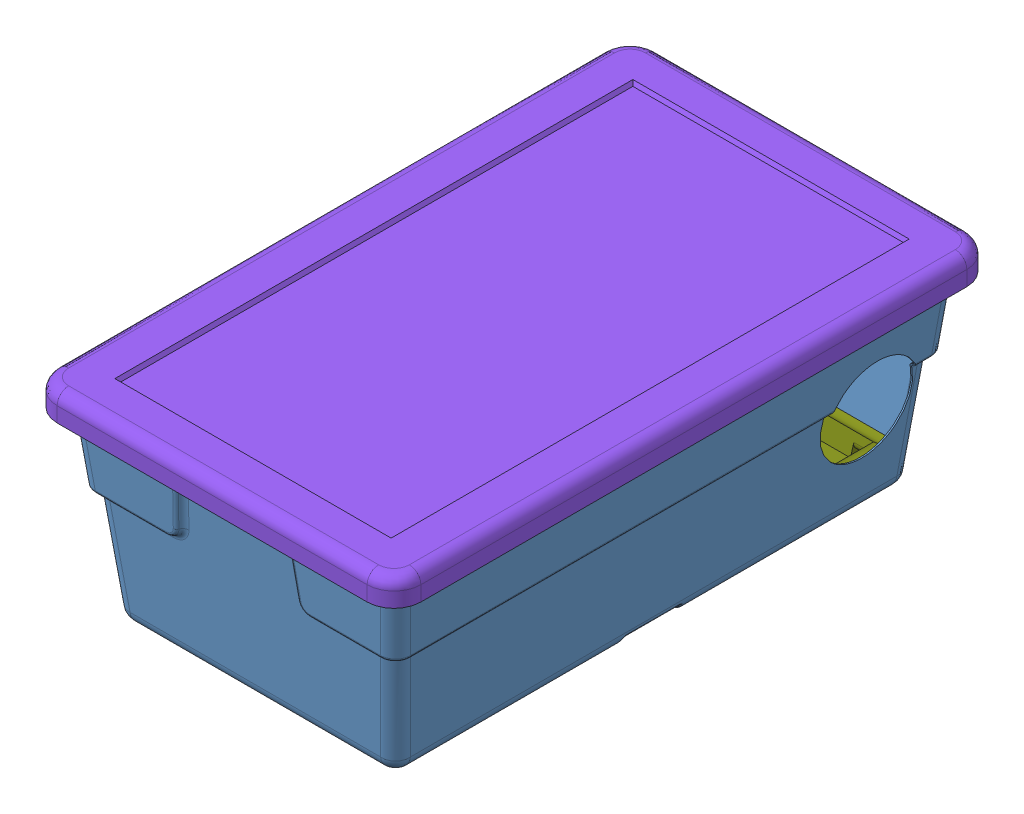
SolidWorks assembly electronics_box, configuration Default. Lengths in mm.
Overall size (200.66 116.21 330.83).
278 component instances, 62 part files, 7 mates.
Components (placement in the parent):
- sterilite_box-1: sterilite_box [Default] at (6.4065 -41.9824 -170.8478) size (195.22 114.3 325.39)
- electronics_tray-1: electronics_tray [Default] at (67.0566 -75.9526 -72.8113) x (0 0 1) z (-1 0 0) size (203.2 36.13 152.4)
  - ibt2_assembly-1: ibt2_assembly [Default] at (25.1982 40.7289 22.1019) size (49.66 21.28 49.78)
    - IBT2_pcb-1: IBT2_pcb [Default] at (-57.2691 7.2367 24.7687) size (49.66 1.57 49.4)
    - header_male_2x4-1: header_male_2x4 [Default] at (4.8115 23.0826 24.5335) x (1 0 0) z (0 -1 0) size (10.16 5.08 10.92)
      - header_pin_base_2x4-1: header_pin_base_2x4 [Default] at (-49.9521 21.6346 11.7311) size (10.16 5.08 2.54)
      - header_pin-1: header_pin [Default] at (-56.3021 22.9046 6.0161) size (0.64 0.64 10.92)
      - header_pin-2: header_pin [Default] at (-56.3021 20.3646 6.0161) size (0.64 0.64 10.92)
      - header_pin-3: header_pin [Default] at (-53.7621 22.9046 6.0161) size (0.64 0.64 10.92)
      - header_pin-4: header_pin [Default] at (-53.7621 20.3646 6.0161) size (0.64 0.64 10.92)
      - header_pin-5: header_pin [Default] at (-51.2221 22.9046 6.0161) size (0.64 0.64 10.92)
      - header_pin-6: header_pin [Default] at (-51.2221 20.3646 6.0161) size (0.64 0.64 10.92)
      - header_pin-7: header_pin [Default] at (-48.6821 22.9046 6.0161) size (0.64 0.64 10.92)
      - header_pin-8: header_pin [Default] at (-48.6821 20.3646 6.0161) size (0.64 0.64 10.92)
    - AMP_screw-terminal_2POS_large-1: AMP_screw-terminal_2POS_large [Default] at (-57.2056 17.0115 0.4662) x (-1 0 0) z (0 0 -1) size (10.66 17 9)
    - AMP_screw-terminal_2POS_large-2: AMP_screw-terminal_2POS_large [Default] at (-47.0456 17.0115 0.4662) x (-1 0 0) z (0 0 -1) size (10.66 17 9)
    - cap_5mm_pitch-1: cap_5mm_pitch [Default] at (-68.3924 8.8115 4.7662) size (10.16 19.69 10.16)
    - d2pak-1: d2pak [Default] at (-63.2409 8.7779 25.6248) x (1 0 0) z (0 0.999978 0.006671) size (9.87 15.09 4.26)
    - d2pak-2: d2pak [Default] at (-52.336 8.7779 25.6248) x (1 0 0) z (0 0.999978 0.006671) size (9.87 15.09 4.26)
    - SOIC20 wide-1: SOIC20 wide [Default] at (-39.9304 8.5615 36.0347) x (1 0 0) z (0 1 0) size (13 10.17 2.01)
    - cap_0805-1: cap_0805 [Default] at (-38.0286 9.3449 27.3468) x (1 0 0) z (0 -1 0) size (2.03 1.32 0.56)
    - resistor_0805-1: resistor_0805 [Default] at (-48.3156 9.3449 41.6216) x (0 0 -1) z (0 -1 0) size (2.03 1.32 0.56)
    - resistor_0805-2: resistor_0805 [Default] at (-50.4517 9.3449 41.6216) x (0 0 -1) z (0 -1 0) size (2.03 1.32 0.56)
    - resistor_0805-3: resistor_0805 [Default] at (-52.5879 9.3449 41.6216) x (0 0 -1) z (0 -1 0) size (2.03 1.32 0.56)
    - resistor_0805-4: resistor_0805 [Default] at (-54.724 9.3449 41.6216) x (0 0 -1) z (0 -1 0) size (2.03 1.32 0.56)
    - resistor_0805-5: resistor_0805 [Default] at (-56.8602 9.3449 41.6216) x (0 0 -1) z (0 -1 0) size (2.03 1.32 0.56)
    - resistor_0805-6: resistor_0805 [Default] at (-58.9963 9.3449 41.6216) x (0 0 -1) z (0 -1 0) size (2.03 1.32 0.56)
    - resistor_0805-7: resistor_0805 [Default] at (-61.1324 9.3449 41.6216) x (0 0 -1) z (0 -1 0) size (2.03 1.32 0.56)
    - resistor_0805-8: resistor_0805 [Default] at (-63.2686 9.3449 41.6216) x (0 0 -1) z (0 -1 0) size (2.03 1.32 0.56)
  - ibt2_assembly-2: ibt2_assembly [Default] at (-89.34 40.7289 121.0422) x (-1 0 0) z (0 0 -1) size (49.66 21.28 49.78)
    - IBT2_pcb-1: IBT2_pcb [Default] at (-57.2691 7.2367 24.7687) size (49.66 1.57 49.4)
    - header_male_2x4-1: header_male_2x4 [Default] at (4.8115 23.0826 24.5335) x (1 0 0) z (0 -1 0) size (10.16 5.08 10.92)
      - header_pin_base_2x4-1: header_pin_base_2x4 [Default] at (-49.9521 21.6346 11.7311) size (10.16 5.08 2.54)
      - header_pin-1: header_pin [Default] at (-56.3021 22.9046 6.0161) size (0.64 0.64 10.92)
      - header_pin-2: header_pin [Default] at (-56.3021 20.3646 6.0161) size (0.64 0.64 10.92)
      - header_pin-3: header_pin [Default] at (-53.7621 22.9046 6.0161) size (0.64 0.64 10.92)
      - header_pin-4: header_pin [Default] at (-53.7621 20.3646 6.0161) size (0.64 0.64 10.92)
      - header_pin-5: header_pin [Default] at (-51.2221 22.9046 6.0161) size (0.64 0.64 10.92)
      - header_pin-6: header_pin [Default] at (-51.2221 20.3646 6.0161) size (0.64 0.64 10.92)
      - header_pin-7: header_pin [Default] at (-48.6821 22.9046 6.0161) size (0.64 0.64 10.92)
      - header_pin-8: header_pin [Default] at (-48.6821 20.3646 6.0161) size (0.64 0.64 10.92)
    - AMP_screw-terminal_2POS_large-1: AMP_screw-terminal_2POS_large [Default] at (-57.2056 17.0115 0.4662) x (-1 0 0) z (0 0 -1) size (10.66 17 9)
    - AMP_screw-terminal_2POS_large-2: AMP_screw-terminal_2POS_large [Default] at (-47.0456 17.0115 0.4662) x (-1 0 0) z (0 0 -1) size (10.66 17 9)
    - cap_5mm_pitch-1: cap_5mm_pitch [Default] at (-68.3924 8.8115 4.7662) size (10.16 19.69 10.16)
    - d2pak-1: d2pak [Default] at (-63.2409 8.7779 25.6248) x (1 0 0) z (0 0.999978 0.006671) size (9.87 15.09 4.26)
    - d2pak-2: d2pak [Default] at (-52.336 8.7779 25.6248) x (1 0 0) z (0 0.999978 0.006671) size (9.87 15.09 4.26)
    - SOIC20 wide-1: SOIC20 wide [Default] at (-39.9304 8.5615 36.0347) x (1 0 0) z (0 1 0) size (13 10.17 2.01)
    - cap_0805-1: cap_0805 [Default] at (-38.0286 9.3449 27.3468) x (1 0 0) z (0 -1 0) size (2.03 1.32 0.56)
    - resistor_0805-1: resistor_0805 [Default] at (-48.3156 9.3449 41.6216) x (0 0 -1) z (0 -1 0) size (2.03 1.32 0.56)
    - resistor_0805-2: resistor_0805 [Default] at (-50.4517 9.3449 41.6216) x (0 0 -1) z (0 -1 0) size (2.03 1.32 0.56)
    - resistor_0805-3: resistor_0805 [Default] at (-52.5879 9.3449 41.6216) x (0 0 -1) z (0 -1 0) size (2.03 1.32 0.56)
    - resistor_0805-4: resistor_0805 [Default] at (-54.724 9.3449 41.6216) x (0 0 -1) z (0 -1 0) size (2.03 1.32 0.56)
    - resistor_0805-5: resistor_0805 [Default] at (-56.8602 9.3449 41.6216) x (0 0 -1) z (0 -1 0) size (2.03 1.32 0.56)
    - resistor_0805-6: resistor_0805 [Default] at (-58.9963 9.3449 41.6216) x (0 0 -1) z (0 -1 0) size (2.03 1.32 0.56)
    - resistor_0805-7: resistor_0805 [Default] at (-61.1324 9.3449 41.6216) x (0 0 -1) z (0 -1 0) size (2.03 1.32 0.56)
    - resistor_0805-8: resistor_0805 [Default] at (-63.2686 9.3449 41.6216) x (0 0 -1) z (0 -1 0) size (2.03 1.32 0.56)
  - Arduino_mega-1: Arduino_mega [Default] at (5.4045 37.4555 130.5264) x (0 0 1) z (0 1 0) size (107.7 53.34 12.38)
    - Arduino_mega-1: Arduino_mega [Default] at (-98.4513 -6.297 10.51) size (101.6 53.34 1.59)
    - USB-jack-1: USB-jack [Default] at (-104.5473 25.6308 12.0975) size (16.46 12.14 10.79)
    - DC-jack-1: DC-jack [Default] at (-99.9245 -2.5632 12.0975) x (0 1 0) z (0 0 -1) size (8.79 13.59 10.72)
    - header_8-pin-1: header_8-pin [Default] at (-53.7727 -5.0778 12.0975) size (20.32 2.54 8.56)
    - header_8-pin-2: header_8-pin [Default] at (-30.6587 -5.0778 12.0975) size (20.32 2.54 8.56)
    - header_8-pin-3: header_8-pin [Default] at (-8.0781 -5.0778 12.0975) size (20.32 2.54 8.56)
    - header_8-pin-4: header_8-pin [Default] at (-35.7895 43.0044 12.0975) size (20.32 2.54 8.56)
    - header_8-pin-5: header_8-pin [Default] at (-13.1835 43.0044 12.0975) size (20.32 2.54 8.56)
    - header_10-pin-1: header_10-pin [Default] at (-58.0145 43.0044 12.0975) size (25.4 2.54 8.56)
    - header_36-pin-1: header_36-pin [Default] at (-0.5343 43.0298 12.0975) x (0 1 0) z (0 0 1) size (45.72 5.08 8.56)
  - arduino uno-1: arduino uno [Default] at (57.5276 49.6156 28.9001) x (-1 0 0) z (0 0 -1) size (53.34 15.25 74.97)
    - unoboard blue-1: unoboard blue [Default] at origin size (53.34 1.65 68.58)
    - 47uf CAP Dcase-1: 47uf CAP Dcase [Default] at (-9.4141 0 -18.4991) x (0 0 -1) z (1 0 0) size (6.6 5.81 8)
    - USB type b-1: USB type b [Default] at (-38.02 0.43 6.35) size (13.72 15.2 16.54)
      - USB SHELL-1: USB SHELL [Default] at origin size (13.72 15.2 16.54)
      - USB core-1: USB core [Default] at origin size (11.3 10.68 15.75)
      - usb top contact-1: usb top contact [Default] at (1.25 6.09 -0.38) size (1 9.67 13.76)
      - usb btm contact-1: usb btm contact [Default] at (1.25 4.41 -0.38) size (1 6.84 11.76)
      - usb btm contact-2: usb btm contact [Default] at (-1.25 4.41 -0.38) size (1 6.84 11.76)
      - usb top contact-2: usb top contact [Default] at (-1.25 6.09 -0.38) size (1 9.67 13.76)
    - power jack-1: power jack [Default] at (-7.675 0 1.905) size (11.2 15.2 15.9)
    - 47uf CAP Dcase-2: 47uf CAP Dcase [Default] at (-9.4141 0 -25.7132) x (0 0 -1) z (1 0 0) size (6.6 5.81 8)
    - crystal-1: crystal [Default] at (-26.162 0 -18.923) x (1 0 0) z (0 0 -1) size (4 5 11)
    - 2pin_header__02-1: 2pin_header__02 [Default] at (-46.23 0 -15.75) size (5 11.75 2.54)
    - nano - reg-1: nano - reg [Default] at (-17.399 0 -7.747) size (6.5 1.69 8.3)
    - led-1: led [Default] at (-34.29 0 -27.94) x (0 0 1) z (-1 0 0) size (4 0.86 1.35)
    - 2pin_header__02-2: 2pin_header__02 [Default] at (-30.43 0 -64.91) x (0 0 1) z (-1 0 0) size (5 11.75 2.54)
    - dip28-1: dip28 [Default] at (-16.383 1.5 -46.355) x (0 0 -1) z (1 0 0) size (35.48 7.37 10.1)
      - dip28-1: dip28 [Default] at origin size (35.48 2.8 10.1)
      - dip socket pin-1: dip socket pin [Default] at (16.51 2.8 -3.81) size (1.7 7.37 1.7)
      - dip socket pin-2: dip socket pin [Default] at (16.51 2.8 3.81) size (1.7 7.37 1.7)
      - dip socket pin-3: dip socket pin [Default] at (13.97 2.8 -3.81) size (1.7 7.37 1.7)
      - dip socket pin-4: dip socket pin [Default] at (13.97 2.8 3.81) size (1.7 7.37 1.7)
      - dip socket pin-5: dip socket pin [Default] at (11.43 2.8 -3.81) size (1.7 7.37 1.7)
      - dip socket pin-6: dip socket pin [Default] at (11.43 2.8 3.81) size (1.7 7.37 1.7)
      - dip socket pin-7: dip socket pin [Default] at (8.89 2.8 -3.81) size (1.7 7.37 1.7)
      - dip socket pin-8: dip socket pin [Default] at (8.89 2.8 3.81) size (1.7 7.37 1.7)
      - dip socket pin-9: dip socket pin [Default] at (6.35 2.8 -3.81) size (1.7 7.37 1.7)
      - dip socket pin-10: dip socket pin [Default] at (6.35 2.8 3.81) size (1.7 7.37 1.7)
      - dip socket pin-11: dip socket pin [Default] at (3.81 2.8 -3.81) size (1.7 7.37 1.7)
      - dip socket pin-12: dip socket pin [Default] at (3.81 2.8 3.81) size (1.7 7.37 1.7)
      - dip socket pin-13: dip socket pin [Default] at (1.27 2.8 -3.81) size (1.7 7.37 1.7)
      - dip socket pin-14: dip socket pin [Default] at (1.27 2.8 3.81) size (1.7 7.37 1.7)
      - dip socket pin-15: dip socket pin [Default] at (-1.27 2.8 -3.81) size (1.7 7.37 1.7)
      - dip socket pin-16: dip socket pin [Default] at (-1.27 2.8 3.81) size (1.7 7.37 1.7)
      - dip socket pin-17: dip socket pin [Default] at (-3.81 2.8 -3.81) size (1.7 7.37 1.7)
      - dip socket pin-18: dip socket pin [Default] at (-3.81 2.8 3.81) size (1.7 7.37 1.7)
      - dip socket pin-19: dip socket pin [Default] at (-6.35 2.8 -3.81) size (1.7 7.37 1.7)
      - dip socket pin-20: dip socket pin [Default] at (-6.35 2.8 3.81) size (1.7 7.37 1.7)
      - dip socket pin-21: dip socket pin [Default] at (-8.89 2.8 -3.81) size (1.7 7.37 1.7)
      - dip socket pin-22: dip socket pin [Default] at (-8.89 2.8 3.81) size (1.7 7.37 1.7)
      - dip socket pin-23: dip socket pin [Default] at (-11.43 2.8 -3.81) size (1.7 7.37 1.7)
      - dip socket pin-24: dip socket pin [Default] at (-11.43 2.8 3.81) size (1.7 7.37 1.7)
      - dip socket pin-25: dip socket pin [Default] at (-13.97 2.8 -3.81) size (1.7 7.37 1.7)
      - dip socket pin-26: dip socket pin [Default] at (-13.97 2.8 3.81) size (1.7 7.37 1.7)
      - dip socket pin-27: dip socket pin [Default] at (-16.51 2.8 -3.81) size (1.7 7.37 1.7)
      - dip socket pin-28: dip socket pin [Default] at (-16.51 2.8 3.81) size (1.7 7.37 1.7)
    - 2pin_header__02-3: 2pin_header__02 [Default] at (-27.89 0 -64.91) x (0 0 1) z (-1 0 0) size (5 11.75 2.54)
    - 2pin_header__02-4: 2pin_header__02 [Default] at (-25.35 0 -64.91) x (0 0 1) z (-1 0 0) size (5 11.75 2.54)
    - 2pin_header__02-5: 2pin_header__02 [Default] at (-46.23 0 -18.29) size (5 11.75 2.54)
    - 2pin_header__02-6: 2pin_header__02 [Default] at (-46.23 0 -20.83) size (5 11.75 2.54)
    - atmega16u2-1: atmega16u2 [Default] at (-34.671 0.06 -20) x (1 0 0) z (0 0 -1) size (5.5 1.01 5.5)
    - led-2: led [Default] at (-36.83 0 -27.94) x (0 0 1) z (-1 0 0) size (4 0.86 1.35)
    - led-3: led [Default] at (-42.037 0 -27.94) x (0 0 1) z (-1 0 0) size (4 0.86 1.35)
    - led-4: led [Default] at (-36.576 0 -58.42) x (0 0 1) z (-1 0 0) size (4 0.86 1.35)
    - 8 PORT HEADER-3: 8 PORT HEADER [Default] at (-50.8 0 -45.72) x (0 0 -1) z (1 0 0) size (20.32 10.51 2.41)
    - 8 PORT HEADER-4: 8 PORT HEADER [Default] at (-2.54 0 -27.94) x (0 0 -1) z (1 0 0) size (20.32 10.51 2.41)
    - 6 PORT HEADER-3: 6 PORT HEADER [Default] at (-2.54 0 -50.8) x (0 0 -1) z (1 0 0) size (15.24 10.51 2.41)
    - 10 PORT HEADER-1: 10 PORT HEADER [Default] at (-50.8 0 -18.796) x (0 0 -1) z (1 0 0) size (25.4 10.51 2.41)
    - ATMEL328P-1: ATMEL328P [Default] at (-16.383 4.3 -46.355) x (0 0 -1) z (1 0 0) size (35 7.27 7.87)
    - 102 RESISTOR PACK-1: 102 RESISTOR PACK [Default] at (-33.782 0 -58.42) size (3.2 0.46 3)
    - 102 RESISTOR PACK-2: 102 RESISTOR PACK [Default] at (-39.37 0 -27.94) size (3.2 0.46 3)
    - 103 RESISTOR PACK-3: 103 RESISTOR PACK [Default] at (-23.876 0 -27.94) size (3.2 0.46 3)
    - 220 RESISTOR PACK-1: 220 RESISTOR PACK [Default] at (-36.83 0 -12.827) size (3.2 0.46 3)
    - 16mhz crystal - measured-1: 16mhz crystal - measured [Default] at (-24.892 0 -41.275) x (0 0 -1) z (1 0 0) size (3.4 0.8 2)
    - PADS001-1: PADS001 [Default] at (-39.878 0.1 -18.288) x (-1 0 0) z (0 0 1) size (4.54 0.1 4.54)
    - 603 cap on pad-1: 603 cap on pad [Default] at (-44.45 0 -27.94) x (0 0 -1) z (1 0 0) size (2.76 0.9 1.12)
    - ssot3-1: ssot3 [Default] at (-26.5 0 -8.128) x (-1 0 0) z (0 0 -1) size (3 1.13 3.09)
    - mf-msmf050-2-1: mf-msmf050-2 [Default] at (-26.5 0 -4.064) size (5.77 1.02 3.72)
    - 603 cap on pad-2: 603 cap on pad [Default] at (-29.845 0 -27.94) x (0 0 -1) z (1 0 0) size (2.76 0.9 1.12)
    - 603 cap on pad-3: 603 cap on pad [Default] at (-31.496 0 -27.94) x (0 0 -1) z (1 0 0) size (2.76 0.9 1.12)
    - lmv358-1: lmv358 [Default] at (-15.24 0 -21.971) x (0 0 -1) z (1 0 0) size (3.7 1.4 2.9)
    - 603 cap on pad-4: 603 cap on pad [Default] at (-15.24 0 -18.415) size (2.76 0.9 1.12)
    - 603 cap on pad-5: 603 cap on pad [Default] at (-29.845 0 -12.065) x (0 0 1) z (-1 0 0) size (2.76 0.9 1.12)
    - 603 cap on pad-6: 603 cap on pad [Default] at (-29.591 0 -22.352) x (0 0 1) z (-1 0 0) size (2.76 0.9 1.12)
    - 603 cap on pad-7: 603 cap on pad [Default] at (-29.591 0 -16.002) x (0 0 1) z (-1 0 0) size (2.76 0.9 1.12)
    - 603 cap on pad-8: 603 cap on pad [Default] at (-41.91 0 -12.7) x (0 0 1) z (-1 0 0) size (2.76 0.9 1.12)
    - lp2985dgkr-1: lp2985dgkr [Default] at (-20.32 0 -19.05) x (0 0 -1) z (1 0 0) size (5.85 1.1 3)
    - cd1206 diode-1: cd1206 diode [Default] at (-27.94 0 -59.436) x (0 0 -1) z (1 0 0) size (2.07 0.96 5)
    - cd1206 diode-2: cd1206 diode [Default] at (-46.228 0 -13.081) x (0 0 1) z (-1 0 0) size (2.07 0.96 5)
    - 603 resistor-1: 603 resistor [Default] at (-29.591 0 -19.05) x (0 0 1) z (-1 0 0) size (2.36 0.61 1.03)
    - blm21-1: blm21 [Default] at (-45.085 0 -7.62) x (0 0 -1) z (1 0 0) size (2.76 0.95 1.32)
    - m7 diode-1: m7 diode [Default] at (-2.794 0 -21.59) x (0 0 -1) z (1 0 0) size (6.66 2.35 2.5)
    - MLC0603-1: MLC0603 [Default] at (-33.655 0 -12.827) x (0 0 -1) z (1 0 0) size (2.36 0.6 1.03)
    - MLC0603-2: MLC0603 [Default] at (-39.37 0 -12.827) x (0 0 -1) z (1 0 0) size (2.36 0.6 1.03)
    - RESET BUTTON-1: RESET BUTTON [Default] at (-49.403 0 -6.35) size (6.2 3.1 9.6)
      - RESET CORE-1: RESET CORE [Default] at (0 0.1 0) x (-1 0 0) z (0 0 -1) size (6.2 3.1 9.6)
      - RESET-1: RESET [Default] at (0 0.1 0) x (0 0 1) z (-1 0 0) size (7.3 2 6.2)
    - 603 cap on pad-9: 603 cap on pad [Default] at (-15.24 0 -25.625) size (2.76 0.9 1.12)
  - electronics_tray_tray-1: electronics_tray_tray [Default] at origin size (203.2 13.95 152.4)
  - m3x6mm_cap_screw-1: m3x6mm_cap_screw [92095A179] at (-11.9414 51.1904 27.3507) x (-0.837169 0 -0.546944) z (0 1 0) size (5.7 5.7 7.77)
  - bms_assembly-1: bms_assembly [Default] at (83.3041 41.8308 46.3558) x (0 0 -1) z (0 1 0) size (88.9 53.34 22.95)
    - bms_board-1: bms_board [Default] at (-80.72 -27.381 18.8348) size (88.9 53.34 1.57)
    - AMP_screw-terminal_2POS_large-1: AMP_screw-terminal_2POS_large [Default] at (-79.94 10.719 28.6096) x (0 -1 0) z (-1 0 0) size (10.66 17 9)
    - AMP_screw-terminal_2POS_large-2: AMP_screw-terminal_2POS_large [Default] at (-79.94 0.559 28.6096) x (0 -1 0) z (-1 0 0) size (10.66 17 9)
    - B4B-XH-Apart-1: B4B-XH-Apart [Default] at (-77.791 -14.995 20.4096) x (0 1 0) z (1 0 0) size (12.4 10.4 5.75)
    - header_male_1x10-1: header_male_1x10 [Default] at (49.0022 32.4877 36.1995) x (0 1 0) z (0 0 1) size (2.54 25.4 10.92)
      - header_pin-1: header_pin [Default] at (-57.3287 73.639 -25.2387) size (0.64 0.64 10.92)
      - header_pin_base_single-1: header_pin_base_single [Default] at (-58.5987 72.369 -19.9047) size (2.54 2.54 2.54)
      - header_pin_base_single-2: header_pin_base_single [Default] at (-58.5987 69.829 -19.9047) size (2.54 2.54 2.54)
      - header_pin_base_single-3: header_pin_base_single [Default] at (-58.5987 67.289 -19.9047) size (2.54 2.54 2.54)
      - header_pin_base_single-4: header_pin_base_single [Default] at (-58.5987 64.749 -19.9047) size (2.54 2.54 2.54)
      - header_pin_base_single-5: header_pin_base_single [Default] at (-58.5987 62.209 -19.9047) size (2.54 2.54 2.54)
      - header_pin_base_single-6: header_pin_base_single [Default] at (-58.5987 59.669 -19.9047) size (2.54 2.54 2.54)
      - header_pin-2: header_pin [Default] at (-57.3287 71.099 -25.2387) size (0.64 0.64 10.92)
      - header_pin-3: header_pin [Default] at (-57.3287 68.559 -25.2387) size (0.64 0.64 10.92)
      - header_pin-4: header_pin [Default] at (-57.3287 66.019 -25.2387) size (0.64 0.64 10.92)
      - header_pin-5: header_pin [Default] at (-57.3287 63.479 -25.2387) size (0.64 0.64 10.92)
      - header_pin-6: header_pin [Default] at (-57.3287 60.939 -25.2387) size (0.64 0.64 10.92)
      - header_pin-7: header_pin [Default] at (-57.3287 58.399 -25.2387) size (0.64 0.64 10.92)
      - header_pin-8: header_pin [Default] at (-57.3287 55.859 -25.2387) size (0.64 0.64 10.92)
      - header_pin_base_single-7: header_pin_base_single [Default] at (-58.5987 57.129 -19.9047) size (2.54 2.54 2.54)
      - header_pin_base_single-8: header_pin_base_single [Default] at (-58.5987 54.589 -19.9047) size (2.54 2.54 2.54)
      - header_pin_base_single-9: header_pin_base_single [Default] at (-58.5987 52.049 -19.9047) size (2.54 2.54 2.54)
      - header_pin_base_single-10: header_pin_base_single [Default] at (-58.5987 49.509 -19.9047) size (2.54 2.54 2.54)
      - header_pin-9: header_pin [Default] at (-57.3287 53.319 -25.2387) size (0.64 0.64 10.92)
      - header_pin-10: header_pin [Default] at (-57.3287 50.779 -25.2387) size (0.64 0.64 10.92)
    - header_male_1x8-1: header_male_1x8 [Default] at (-84.3058 -33.9097 36.1995) x (0 -1 0) z (0 0 1) size (2.54 20.32 10.92)
      - header_pin-1: header_pin [Default] at (-57.3287 73.639 -25.2387) size (0.64 0.64 10.92)
      - header_pin_base_single-1: header_pin_base_single [Default] at (-58.5987 72.369 -19.9047) size (2.54 2.54 2.54)
      - header_pin_base_single-2: header_pin_base_single [Default] at (-58.5987 69.829 -19.9047) size (2.54 2.54 2.54)
      - header_pin_base_single-3: header_pin_base_single [Default] at (-58.5987 67.289 -19.9047) size (2.54 2.54 2.54)
      - header_pin_base_single-4: header_pin_base_single [Default] at (-58.5987 64.749 -19.9047) size (2.54 2.54 2.54)
      - header_pin_base_single-5: header_pin_base_single [Default] at (-58.5987 62.209 -19.9047) size (2.54 2.54 2.54)
      - header_pin_base_single-6: header_pin_base_single [Default] at (-58.5987 59.669 -19.9047) size (2.54 2.54 2.54)
      - header_pin-2: header_pin [Default] at (-57.3287 71.099 -25.2387) size (0.64 0.64 10.92)
      - header_pin-3: header_pin [Default] at (-57.3287 68.559 -25.2387) size (0.64 0.64 10.92)
      - header_pin-4: header_pin [Default] at (-57.3287 66.019 -25.2387) size (0.64 0.64 10.92)
      - header_pin-5: header_pin [Default] at (-57.3287 63.479 -25.2387) size (0.64 0.64 10.92)
      - header_pin-6: header_pin [Default] at (-57.3287 60.939 -25.2387) size (0.64 0.64 10.92)
      - header_pin-7: header_pin [Default] at (-57.3287 58.399 -25.2387) size (0.64 0.64 10.92)
      - header_pin-8: header_pin [Default] at (-57.3287 55.859 -25.2387) size (0.64 0.64 10.92)
      - header_pin_base_single-7: header_pin_base_single [Default] at (-58.5987 57.129 -19.9047) size (2.54 2.54 2.54)
      - header_pin_base_single-8: header_pin_base_single [Default] at (-58.5987 54.589 -19.9047) size (2.54 2.54 2.54)
    - header_male_1x8-2: header_male_1x8 [Default] at (-102.0858 -82.1697 36.1995) x (0 -1 0) z (0 0 1) size (2.54 20.32 10.92)
      - header_pin-1: header_pin [Default] at (-57.3287 73.639 -25.2387) size (0.64 0.64 10.92)
      - header_pin_base_single-1: header_pin_base_single [Default] at (-58.5987 72.369 -19.9047) size (2.54 2.54 2.54)
      - header_pin_base_single-2: header_pin_base_single [Default] at (-58.5987 69.829 -19.9047) size (2.54 2.54 2.54)
      - header_pin_base_single-3: header_pin_base_single [Default] at (-58.5987 67.289 -19.9047) size (2.54 2.54 2.54)
      - header_pin_base_single-4: header_pin_base_single [Default] at (-58.5987 64.749 -19.9047) size (2.54 2.54 2.54)
      - header_pin_base_single-5: header_pin_base_single [Default] at (-58.5987 62.209 -19.9047) size (2.54 2.54 2.54)
      - header_pin_base_single-6: header_pin_base_single [Default] at (-58.5987 59.669 -19.9047) size (2.54 2.54 2.54)
      - header_pin-2: header_pin [Default] at (-57.3287 71.099 -25.2387) size (0.64 0.64 10.92)
      - header_pin-3: header_pin [Default] at (-57.3287 68.559 -25.2387) size (0.64 0.64 10.92)
      - header_pin-4: header_pin [Default] at (-57.3287 66.019 -25.2387) size (0.64 0.64 10.92)
      - header_pin-5: header_pin [Default] at (-57.3287 63.479 -25.2387) size (0.64 0.64 10.92)
      - header_pin-6: header_pin [Default] at (-57.3287 60.939 -25.2387) size (0.64 0.64 10.92)
      - header_pin-7: header_pin [Default] at (-57.3287 58.399 -25.2387) size (0.64 0.64 10.92)
      - header_pin-8: header_pin [Default] at (-57.3287 55.859 -25.2387) size (0.64 0.64 10.92)
      - header_pin_base_single-7: header_pin_base_single [Default] at (-58.5987 57.129 -19.9047) size (2.54 2.54 2.54)
      - header_pin_base_single-8: header_pin_base_single [Default] at (-58.5987 54.589 -19.9047) size (2.54 2.54 2.54)
    - header_male_1x6-1: header_male_1x6 [Default] at (27.4122 80.7477 36.1995) x (0 1 0) z (0 0 1) size (2.54 15.24 10.92)
      - header_pin-1: header_pin [Default] at (-57.3287 73.639 -25.2387) size (0.64 0.64 10.92)
      - header_pin_base_single-1: header_pin_base_single [Default] at (-58.5987 72.369 -19.9047) size (2.54 2.54 2.54)
      - header_pin_base_single-2: header_pin_base_single [Default] at (-58.5987 69.829 -19.9047) size (2.54 2.54 2.54)
      - header_pin_base_single-3: header_pin_base_single [Default] at (-58.5987 67.289 -19.9047) size (2.54 2.54 2.54)
      - header_pin_base_single-4: header_pin_base_single [Default] at (-58.5987 64.749 -19.9047) size (2.54 2.54 2.54)
      - header_pin_base_single-5: header_pin_base_single [Default] at (-58.5987 62.209 -19.9047) size (2.54 2.54 2.54)
      - header_pin_base_single-6: header_pin_base_single [Default] at (-58.5987 59.669 -19.9047) size (2.54 2.54 2.54)
      - header_pin-2: header_pin [Default] at (-57.3287 71.099 -25.2387) size (0.64 0.64 10.92)
      - header_pin-3: header_pin [Default] at (-57.3287 68.559 -25.2387) size (0.64 0.64 10.92)
      - header_pin-4: header_pin [Default] at (-57.3287 66.019 -25.2387) size (0.64 0.64 10.92)
      - header_pin-5: header_pin [Default] at (-57.3287 63.479 -25.2387) size (0.64 0.64 10.92)
      - header_pin-6: header_pin [Default] at (-57.3287 60.939 -25.2387) size (0.64 0.64 10.92)
    - AMP_screw-terminal_8POS_small-1: AMP_screw-terminal_8POS_small [Default] at (4.7256 -13.9952 30.4096) x (0 1 0) z (0 0 1) size (20.78 6.55 13.4)
  - mainboard_assembly-1: mainboard_assembly [Default] at (75.8522 66.1104 104.8773) size (53.34 22.95 96.52)
    - AMP_screw-terminal_2POS_large-1: AMP_screw-terminal_2POS_large [Default] at (-33.2598 4.3173 21.1598) size (10.66 17 9)
    - mainboard_pcb-1: mainboard_pcb [Default] at (-23.6078 -5.4575 23.8448) x (0 0 -1) z (1 0 0) size (96.52 1.57 53.34)
    - AMP_screw-terminal_2POS_large-2: AMP_screw-terminal_2POS_large [Default] at (-53.5798 4.3173 21.1598) size (10.66 17 9)
    - AMP_screw-terminal_2POS_large-3: AMP_screw-terminal_2POS_large [Default] at (-43.4198 4.3173 21.1598) size (10.66 17 9)
    - header_male_1x18-1: header_male_1x18 [Default] at (4.3112 11.9071 -36.0239) x (0 0 -1) z (0 1 0) size (2.54 45.72 10.92)
      - header_pin-1: header_pin [Default] at (-57.3287 73.639 -25.2387) size (0.64 0.64 10.92)
      - header_pin_base_single-1: header_pin_base_single [Default] at (-58.5987 72.369 -19.9047) size (2.54 2.54 2.54)
      - header_pin_base_single-2: header_pin_base_single [Default] at (-58.5987 69.829 -19.9047) size (2.54 2.54 2.54)
      - header_pin_base_single-3: header_pin_base_single [Default] at (-58.5987 67.289 -19.9047) size (2.54 2.54 2.54)
      - header_pin_base_single-4: header_pin_base_single [Default] at (-58.5987 64.749 -19.9047) size (2.54 2.54 2.54)
      - header_pin_base_single-5: header_pin_base_single [Default] at (-58.5987 62.209 -19.9047) size (2.54 2.54 2.54)
      - header_pin_base_single-6: header_pin_base_single [Default] at (-58.5987 59.669 -19.9047) size (2.54 2.54 2.54)
      - header_pin-2: header_pin [Default] at (-57.3287 71.099 -25.2387) size (0.64 0.64 10.92)
      - header_pin-3: header_pin [Default] at (-57.3287 68.559 -25.2387) size (0.64 0.64 10.92)
      - header_pin-4: header_pin [Default] at (-57.3287 66.019 -25.2387) size (0.64 0.64 10.92)
      - header_pin-5: header_pin [Default] at (-57.3287 63.479 -25.2387) size (0.64 0.64 10.92)
      - header_pin-6: header_pin [Default] at (-57.3287 60.939 -25.2387) size (0.64 0.64 10.92)
      - header_pin-7: header_pin [Default] at (-57.3287 58.399 -25.2387) size (0.64 0.64 10.92)
      - header_pin-8: header_pin [Default] at (-57.3287 55.859 -25.2387) size (0.64 0.64 10.92)
      - header_pin_base_single-7: header_pin_base_single [Default] at (-58.5987 57.129 -19.9047) size (2.54 2.54 2.54)
      - header_pin_base_single-8: header_pin_base_single [Default] at (-58.5987 54.589 -19.9047) size (2.54 2.54 2.54)
      - header_pin_base_single-9: header_pin_base_single [Default] at (-58.5987 52.049 -19.9047) size (2.54 2.54 2.54)
      - header_pin_base_single-10: header_pin_base_single [Default] at (-58.5987 49.509 -19.9047) size (2.54 2.54 2.54)
      - header_pin-9: header_pin [Default] at (-57.3287 53.319 -25.2387) size (0.64 0.64 10.92)
      - header_pin-10: header_pin [Default] at (-57.3287 50.779 -25.2387) size (0.64 0.64 10.92)
      - header_pin-11: header_pin [Default] at (-57.3287 48.239 -25.2387) size (0.64 0.64 10.92)
      - header_pin-12: header_pin [Default] at (-57.3287 45.699 -25.2387) size (0.64 0.64 10.92)
      - header_pin-13: header_pin [Default] at (-57.3287 43.159 -25.2387) size (0.64 0.64 10.92)
      - header_pin-14: header_pin [Default] at (-57.3287 40.619 -25.2387) size (0.64 0.64 10.92)
      - header_pin-15: header_pin [Default] at (-57.3287 38.079 -25.2387) size (0.64 0.64 10.92)
      - header_pin-16: header_pin [Default] at (-57.3287 35.539 -25.2387) size (0.64 0.64 10.92)
      - header_pin-17: header_pin [Default] at (-57.3287 32.999 -25.2387) size (0.64 0.64 10.92)
      - header_pin-18: header_pin [Default] at (-57.3287 30.459 -25.2387) size (0.64 0.64 10.92)
      - header_pin_base_single-11: header_pin_base_single [Default] at (-58.5987 46.969 -19.9047) size (2.54 2.54 2.54)
      - header_pin_base_single-12: header_pin_base_single [Default] at (-58.5987 44.429 -19.9047) size (2.54 2.54 2.54)
      - header_pin_base_single-13: header_pin_base_single [Default] at (-58.5987 41.889 -19.9047) size (2.54 2.54 2.54)
      - header_pin_base_single-14: header_pin_base_single [Default] at (-58.5987 39.349 -19.9047) size (2.54 2.54 2.54)
      - header_pin_base_single-15: header_pin_base_single [Default] at (-58.5987 36.809 -19.9047) size (2.54 2.54 2.54)
      - header_pin_base_single-16: header_pin_base_single [Default] at (-58.5987 34.269 -19.9047) size (2.54 2.54 2.54)
      - header_pin_base_single-17: header_pin_base_single [Default] at (-58.5987 31.729 -19.9047) size (2.54 2.54 2.54)
      - header_pin_base_single-18: header_pin_base_single [Default] at (-58.5987 29.189 -19.9047) size (2.54 2.54 2.54)
  - wire_gnd-bms-main^electronics_tray-1: wire_gnd-bms-main^electronics_tray [Default] at (0 50.7851 -6.0475) x (1 -0.000001 -0.000005) z (0 0.992984 -0.118245) size (37.87 6.32 15) (virtual)
  - wire_gnd-bms-battery^electronics_tray-1: wire_gnd-bms-battery^electronics_tray [Default] at (82.7451 70.4404 124.8958) size (31.16 14.04 136.17) (virtual)
  - wire_gnd-main-BTS^electronics_tray-1: wire_gnd-main-BTS^electronics_tray [Default] at (22.2724 70.4277 124.6371) size (52.12 15.48 13.93) (virtual)
- Sterilite_Lid-1: Sterilite_Lid [Default] at (6.4065 59.6176 -12.868) x (0 0 1) z (-1 0 0) size (330.83 14.61 200.66)
Mates (geometry in assembly coordinates):
- Coincident1: coincident anti-aligned: plane of sterilite_box-1 through (6.4065 -36.3436 -170.8478) normal (0 1 0); plane of electronics_tray-1/electronics_tray_tray-1 through (67.0566 -36.3436 -72.8113) normal (0 -1 0)
- Parallel1: parallel anti-aligned: line of sterilite_box-1 through (-70.9405 -34.5192 -147.8311) axis (0 0 1); line of electronics_tray-1/electronics_tray_tray-1 through (-69.7935 -36.3436 48.0892) axis (0 0 -1)
- Coincident3: coincident: plane of sterilite_box-1 through (6.4065 -41.9824 -170.8478) normal (1 0 0); moEndPointRef_w of electronics_tray-1/electronics_tray_tray-1
- Coincident5: coincident: plane of sterilite_box-1 through (-85.6685 -41.8975 -154.527) normal (0 0.104528 0.994522); line of electronics_tray-1/electronics_tray_tray-1 through (-62.1735 -36.3436 -155.1108) axis (1 0 0)
- Coincident6: coincident anti-aligned: plane of sterilite_box-1 through (6.4065 -41.9824 -170.8478) normal (1 0 0); plane of Sterilite_Lid-1 through (6.4065 59.6176 -12.868) normal (-1 0 0)
- Coincident8: coincident anti-aligned: plane of sterilite_box-1 through (-85.6685 72.3176 143.4772) normal (0 1 0); plane of Sterilite_Lid-1 through (-77.1849 72.3176 135.8109) normal (0 -1 0)
- Coincident9: coincident anti-aligned: plane of sterilite_box-1 through (-76.3676 71.5048 -176.3805) normal (0 0 -1); plane of Sterilite_Lid-1 through (89.9979 72.3176 -176.3805) normal (0 0 1)
